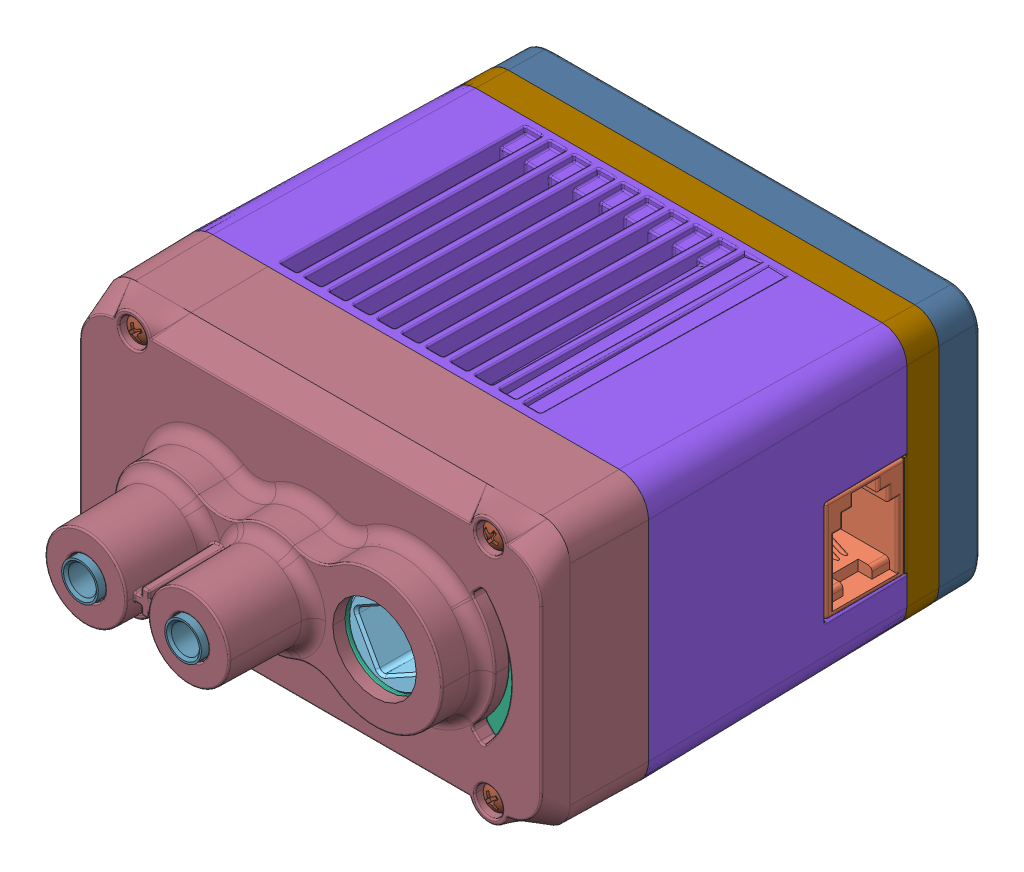
SolidWorks assembly V5 Smart Motor (276-4840), configuration Default. Lengths in mm.
Overall size (59.01 35.33 72.31).
26 component instances, 15 part files, 0 mates.
Components (placement in the parent):
- V5 Smart Motor (276-4840).step-1: V5 Smart Motor (276-4840).step [Default] at origin size (59.01 35.33 72.31)
  - 276-4840-900 Rev6_Instruction.step-1: 276-4840-900 Rev6_Instruction.step [Default] at (-14.3 0 -17.2) size (52.79 15.94 38.15)
    - 276-4840-901 Rev6.step-1: 276-4840-901 Rev6.step [Default] at (10.75 -10.05 17.8) x (-1 0 0) z (0 0 1) size (49.9 1.6 38.15)
    - 276-4840-902 Rev2.step-1: 276-4840-902 Rev2.step [Default] at (31.25 -9.25 6.2) x (0 0 -1) z (0 -1 0) size (10.35 11.39 15.94)
    - 276-4840-022 Rev4.step-1: 276-4840-022 Rev4.step [Default] at (31.25 -9.25 6.2) x (0 0 -1) z (1 0 0) size (10.26 9.1 5.51)
  - 276-4840-110 Rev10_Instruction.step-1: 276-4840-110 Rev10_Instruction.step [Default] at (12.7 0 14.7) size (35.33 35.33 31.1)
    - 276-4840-061 Rev7_Ring_Gear_Fixed01 .6 Rev3.step-1: 276-4840-061 Rev7_Ring_Gear_Fixed01 .6 Rev3.step [Default] at origin size (28.79 28.39 24.6)
    - 276-4840-018 Rev6.step-1: 276-4840-018 Rev6.step [Default] at (0 0 6.7) x (-0.483174 0.875524 0) z (0 0 1) size (26 26 12.3)
    - 276-4840-059 Rev2.step-1: 276-4840-059 Rev2.step [Default] at (0 0 10.3) size (28.4 28.4 8.5)
    - 276-4840-062 Rev1.step-1: 276-4840-062 Rev1.step [Default] at (-12.1353 8.8168 12.3) x (0.956835 -0.290632 0) z (-0.290632 -0.956835 0) size (3.2 6.56 3.2)
    - 276-4840-062 Rev1.step-2: 276-4840-062 Rev1.step [Default] at (12.1353 8.8168 12.3) x (0.978427 0.206591 0) z (0.206591 -0.978427 0) size (3.2 6.56 3.2)
    - 276-4840-062 Rev1.step-3: 276-4840-062 Rev1.step [Default] at (-12.1353 -8.8168 12.3) x (0.72563 0.688086 0) z (0.688086 -0.72563 0) size (3.2 6.56 3.2)
  - 276-4840-001 Rev38.step-1: 276-4840-001 Rev38.step [Default] at origin size (57.3 33 46.9)
  - 276-4840-005 Rev27.step-1: 276-4840-005 Rev27.step [Default] at (0 0 -17.95) size (56.17 31.87 12.9)
  - 276-4840-004 Rev16.step-1: 276-4840-004 Rev16.step [Default] at (0 0 -19.2) size (56.01 31.71 9.21)
  - 276-4840-015 Rev7.step-1: 276-4840-015 Rev7.step [Default] at (-21.95 14 27.9) x (-0.85131 -0.524663 0) z (-0.524663 0.85131 0) size (3.2 17.55 3.2)
  - 276-4840-015 Rev7.step-2: 276-4840-015 Rev7.step [Default] at (21.95 -14 27.9) x (-0.777574 -0.628792 0) z (-0.628792 0.777574 0) size (3.2 17.55 3.2)
  - 276-4840-015 Rev7.step-3: 276-4840-015 Rev7.step [Default] at (21.95 14 27.9) x (0.476859 0.87898 0) z (0.87898 -0.476859 0) size (3.2 17.55 3.2)
  - 276-4840-009 Rev3.step-1: 276-4840-009 Rev3.step [Default] at (25.45 13.5 15.7) x (0.19987 -0.979823 0) z (-0.979823 -0.19987 0) size (3.4 41.31 4.34)
  - 276-4840-009 Rev3.step-2: 276-4840-009 Rev3.step [Default] at (-25.45 -13.5 15.7) x (-0.998855 0.047836 0) z (0.047836 0.998855 0) size (3.4 41.31 4.34)
  - 276-4840-009 Rev3.step-3: 276-4840-009 Rev3.step [Default] at (25.45 -13.5 15.7) x (-0.975374 0.220559 0) z (0.220559 0.975374 0) size (3.4 41.31 4.34)
  - 276-4840-009 Rev3.step-4: 276-4840-009 Rev3.step [Default] at (-25.45 13.5 15.7) x (-0.922256 0.38658 0) z (0.38658 0.922256 0) size (3.4 41.31 4.34)
  - 276-4840-003 Rev27.step-1: 276-4840-003 Rev27.step [Default] at (0 0 16.2) size (57.3 33 28.01)
  - 276-4840-043 Rev8.step-1: 276-4840-043 Rev8.step [Default] at (-12.7 0 36.2) x (-0.5 -0.866025 0) z (-0.866025 0.5 0) size (6.3 15.2 7.21)
  - 276-4840-043 Rev8.step-2: 276-4840-043 Rev8.step [Default] at (0 0 36.2) x (-0.5 -0.866025 0) z (-0.866025 0.5 0) size (6.3 15.2 7.21)
  - 276-4840-025 Rev19.step-1: 276-4840-025 Rev19.step [Default] at (12.7 0 -22.63) x (-0.993315 0.115437 0) z (0 0 1) size (14.82 14.83 35.18)
